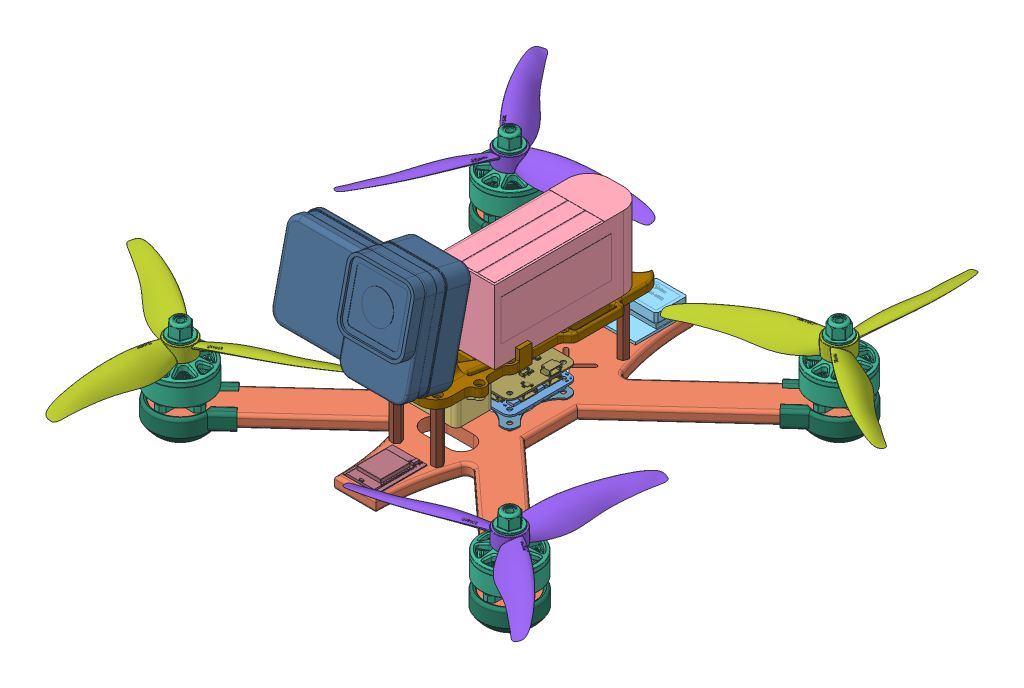
SolidWorks assembly Quad_assem, configuration Default. Lengths in mm.
Overall size (299.08 101.42 318.47).
26 component instances, 15 part files, 57 mates.
Components (placement in the parent):
- 4in1_ESC-1: 4in1_ESC [Default] at (-19.4317 14.4597 116.374) x (-1 0 0) z (0 1 0) size (33 33 7.6)
- Quad-1: Quad [Default] at (-19.4317 0 116.374) x (-1 0 0) z (0 0 -1) size (185.81 6.16 185.81)
- ToF-1: ToF [Default] at (-19.4317 31 146.374) x (1 0 0) z (0 0 -1) size (34.5 13.5 18.5)
- Battery-1: Battery [Default] at (-6 52.75 100.8519) x (0 0 1) z (-1 0 0) size (72.6 35.7 27.2)
- GPS_sam-m8q-2: GPS_sam-m8q [Default] at (-27.0434 7.25 37.7378) size (16.15 7.55 26.25)
- DYS SF2207 Motor.step-1: DYS SF2207 Motor.step [Default] at (60.4714 6 196.277) x (-0.126886 0 -0.991917) z (0.991917 0 -0.126886) size (27.7 33.34 27.7)
- DYS SF2207 Motor.step-2: DYS SF2207 Motor.step [Default] at (60.4714 6 36.4709) x (0.985702 0 -0.1685) z (0.1685 0 0.985702) size (27.7 33.34 27.7)
- DYS SF2207 Motor.step-3: DYS SF2207 Motor.step [Default] at (-99.3348 6 36.4709) x (0.155615 0 0.987818) z (-0.987818 0 0.155615) size (27.7 33.34 27.7)
- DYS SF2207 Motor.step-4: DYS SF2207 Motor.step [Default] at (-99.3348 6 196.277) x (0.148303 0 0.988942) z (-0.988942 0 0.148303) size (27.7 33.34 27.7)
- 50 Prop CW-1: 50 Prop CW [Default] at (60.4714 25.2 36.4709) x (-0.893778 0 0.44851) z (-0.44851 0 -0.893778) size (98.6 8.5 111.89)
- 50 Prop CCW-1: 50 Prop CCW [Default] at (2.1837 28.725 127.366) x (0.945285 0 -0.326246) z (0.326246 0 0.945285) size (98.59 8.5 111.89)
- 50 Prop CCW-2: 50 Prop CCW [Default] at (-50.9884 28.725 -39.7446) x (0.593794 0 0.804617) z (-0.804617 0 0.593794) size (98.59 8.5 111.89)
- 50 Prop CW-2: 50 Prop CW [Default] at (-99.3348 25.2 196.277) x (-0.021995 0 0.999758) z (-0.999758 0 -0.021995) size (98.6 8.5 111.89)
- Quad Top-1: Quad Top [Default] at (-19.4317 31 116.374) x (-1 0 0) z (0 0 -1) size (36.7 13 110.63)
- GOPRO_10_BONES-1: GOPRO_10_BONES [Default] at (-70.9317 42.3222 182.949) x (1 0 0) z (0 0.975758 -0.218854) size (68 37 50)
- Spacer-1: Spacer [Default] at (-9.4317 6 71.374) x (0.702092 0 0.712086) z (-0.712086 0 0.702092) size (5 25 4.33)
- Spacer-2: Spacer [Default] at (-29.4317 6 71.374) x (0.624402 0 0.781104) z (-0.781104 0 0.624402) size (5 25 4.33)
- Spacer-3: Spacer [Default] at (-9.4317 6 161.374) x (0.997584 0 -0.069465) z (0.069465 0 0.997584) size (5 25 4.33)
- Spacer-4: Spacer [Default] at (-29.4317 6 161.374) x (0.991206 0 0.132327) z (-0.132327 0 0.991206) size (5 25 4.33)
- FlightController-1: FlightController [Default] at (-19.4317 21.1634 116.374) x (-1 0 0) z (0 1 0) size (33 33.5 8.12)
- XBee_breakout-1: XBee_breakout [Default] at (-19.5608 6.4115 179.1808) x (-1 0 0) z (0 1 0) size (16.8 24.05 2.88)
- OpticalSensor.step-1: OpticalSensor.step [Default] at (-19.4317 8.6237 116.374) x (0 0 -1) z (0 1 0) size (33 33 6.87)
- Feet-1: Feet [Default] at (60.4714 -1 196.277) x (-0.999023 0 0.044203) z (-0.044203 0 -0.999023) size (35.07 16.09 35.07)
- Feet-2: Feet [Default] at (-99.3348 -1 36.4709) x (0.998911 0 -0.046652) z (0.046652 0 0.998911) size (35.07 16.09 35.07)
- Feet-3: Feet [Default] at (60.4714 -1 36.4709) x (-0.052266 0 0.998633) z (-0.998633 0 -0.052266) size (35.07 16.09 35.07)
- Feet-4: Feet [Default] at (-99.3348 -1 196.277) x (0.04359 0 -0.999049) z (0.999049 0 0.04359) size (35.07 16.09 35.07)
Mates (geometry in assembly coordinates):
- Distance6: distance = 6 mm aligned: plane of Battery-1 through (-6 52.75 100.8519) normal (1 0 0)
- Concentric5: concentric aligned: circle of 4in1_ESC-1; circle of Quad-1
- Concentric6: concentric aligned: circle of 4in1_ESC-1; circle of Quad-1
- Coincident38: coincident anti-aligned: plane of Quad-1 through (-99.3348 6 36.4709) normal (0 1 0); plane of DYS SF2207 Motor.step-1 through (64.4945 6 192.5268) normal (0 -1 0)
- Coincident39: coincident anti-aligned: plane of Quad-1 through (-99.3348 6 36.4709) normal (0 1 0); plane of DYS SF2207 Motor.step-2 through (64.3876 6 40.3327) normal (0 -1 0)
- Coincident40: coincident anti-aligned: plane of Quad-1 through (-99.3348 6 36.4709) normal (0 1 0); plane of DYS SF2207 Motor.step-3 through (-103.2474 6 40.3363) normal (0 -1 0)
- Coincident41: coincident anti-aligned: plane of Quad-1 through (-99.3348 6 36.4709) normal (0 1 0); plane of DYS SF2207 Motor.step-4 through (-103.2759 6 200.1134) normal (0 -1 0)
- Coincident42: coincident anti-aligned: plane of DYS SF2207 Motor.step-1 through (56.3233 25.2 192.978) normal (0 1 0); plane of 50 Prop CCW-1 through (60.4714 25.2 196.277) normal (0 -1 0)
- Coincident43: coincident anti-aligned: plane of DYS SF2207 Motor.step-3 through (-95.0927 25.2 39.6482) normal (0 1 0); plane of 50 Prop CCW-2 through (-99.3348 25.2 36.4709) normal (0 -1 0)
- Coincident44: coincident anti-aligned: plane of DYS SF2207 Motor.step-4 through (-95.1163 25.2 199.4856) normal (0 1 0); plane of 50 Prop CW-2 through (-99.3348 25.2 196.277) normal (0 -1 0)
- Coincident45: coincident anti-aligned: plane of DYS SF2207 Motor.step-2 through (63.593 25.2 32.1877) normal (0 1 0); plane of 50 Prop CW-1 through (60.4714 25.2 36.4709) normal (0 -1 0)
- Concentric15: concentric aligned: cylinder of DYS SF2207 Motor.step-1 through (60.4714 25.2 196.277) axis (0 1 0) radius 2.5; cylinder of 50 Prop CCW-1 through (60.4714 28.7 196.277) axis (0 1 0) radius 2.5
- Concentric16: concentric anti-aligned: cylinder of DYS SF2207 Motor.step-2 through (60.4714 25.2 36.4709) axis (0 1 0) radius 2.5; cylinder of 50 Prop CW-1 through (60.4714 28.7 36.4709) axis (0 -1 0) radius 2.5
- Concentric17: concentric aligned: cylinder of DYS SF2207 Motor.step-3 through (-99.3348 25.2 36.4709) axis (0 1 0) radius 2.5; cylinder of 50 Prop CCW-2 through (-99.3348 28.7 36.4709) axis (0 1 0) radius 2.5
- Concentric18: concentric anti-aligned: cylinder of DYS SF2207 Motor.step-4 through (-99.3348 25.2 196.277) axis (0 1 0) radius 2.5; cylinder of 50 Prop CW-2 through (-99.3348 28.7 196.277) axis (0 -1 0) radius 2.5
- Concentric19: concentric aligned: cylinder of DYS SF2207 Motor.step-3 through (-99.3348 25.2 36.4709) axis (0 1 0) radius 2.5; cylinder of 50 Prop CCW-2 through (-99.3348 28.7 36.4709) axis (0 1 0) radius 2.5
- Coincident53: coincident anti-aligned: plane of ToF-1 through (-8.7317 31 139.624) normal (0 1 0); plane of Quad Top-1 through (-4.1817 31 146.374) normal (0 -1 0)
- Concentric25: concentric aligned: circle of Quad-1; circle of Quad Top-1
- Concentric26: concentric aligned: circle of Quad-1; circle of Quad Top-1
- Coincident57: coincident anti-aligned: plane of Quad-1 through (-99.3348 0 36.4709) normal (0 -1 0)
- Coincident58: coincident anti-aligned: plane of Quad-1 through (-99.3348 6 36.4709) normal (0 1 0); plane of GPS_sam-m8q-2 through (-27.0434 6 37.7378) normal (0 -1 0)
- Parallel1: parallel aligned: plane of Quad-1 through (-10.4317 63.0088 36.374) normal (1 0 0); plane of GPS_sam-m8q-2 through (-11.2684 6 63.5878) normal (1 0 0)
- Concentric27: concentric aligned: circle of Quad-1; circle of DYS SF2207 Motor.step-1
- Concentric28: concentric aligned: circle of Quad-1; circle of DYS SF2207 Motor.step-4
- Concentric29: concentric aligned: circle of Quad-1; circle of DYS SF2207 Motor.step-3
- Concentric30: concentric aligned: circle of Quad-1; circle of DYS SF2207 Motor.step-2
- Concentric31: concentric anti-aligned: circle of Quad Top-1; circle of GOPRO_10_BONES-1
- Distance10: distance = 3 mm aligned: plane of GOPRO_10_BONES-1 through (-22.1817 38.2643 160.2878) normal (-1 0 0); plane of Quad Top-1 through (-25.1817 44 158.374) normal (-1 0 0)
- Concentric32: concentric aligned: circle of Quad-1; circle of Spacer-3
- Concentric33: concentric aligned: circle of Quad-1; circle of Spacer-1
- Concentric34: concentric aligned: circle of Quad-1; circle of Spacer-2
- Concentric35: concentric aligned: circle of Quad-1; circle of Spacer-4
- Coincident60: coincident anti-aligned: plane of Quad-1 through (-99.3348 6 36.4709) normal (0 1 0); plane of Spacer-2 through (-29.4317 6 71.374) normal (0 -1 0)
- Coincident61: coincident anti-aligned: plane of Quad-1 through (-99.3348 6 36.4709) normal (0 1 0); plane of Spacer-4 through (-29.4317 6 161.374) normal (0 -1 0)
- Coincident62: coincident anti-aligned: plane of Quad-1 through (-99.3348 6 36.4709) normal (0 1 0); plane of Spacer-3 through (-9.4317 6 161.374) normal (0 -1 0)
- Coincident63: coincident anti-aligned: plane of Quad-1 through (-99.3348 6 36.4709) normal (0 1 0); plane of Spacer-1 through (-9.4317 6 71.374) normal (0 -1 0)
- Distance13: distance = 6.08 mm anti-aligned: plane of FlightController-1 through (-19.4317 20.5397 116.374) normal (0 -1 0); plane of 4in1_ESC-1 through (-2.9317 14.4597 103.374) normal (0 1 0)
- Concentric42: concentric aligned: circle of 4in1_ESC-1; circle of FlightController-1
- Concentric43: concentric aligned: circle of 4in1_ESC-1; circle of FlightController-1
- Concentric44: concentric anti-aligned: circle of ToF-1; circle of Quad Top-1
- Concentric45: concentric anti-aligned: circle of ToF-1; circle of Quad Top-1
- Coincident78: coincident anti-aligned: plane of Quad-1 through (-99.3348 6 36.4709) normal (0 1 0); plane of XBee_breakout-1 through (-19.5608 6 176.8033) normal (0 -1 0)
- Coincident80: coincident anti-aligned: plane of Quad Top-1 through (-4.1817 31 146.374) normal (0 -1 0); plane of Spacer-3 through (-9.4317 31 161.374) normal (0 1 0)
- Coincident81: coincident anti-aligned: plane of Battery-1 through (-33 35 64.5519) normal (0 -1 0); plane of Quad Top-1 through (-4.1817 35 146.374) normal (0 1 0)
- Parallel6: parallel aligned: plane of XBee_breakout-1 through (-27.9608 6 188.8258) normal (-1 0 0); plane of Quad-1 through (-39.4317 231.245 103.485) normal (-1 0 0)
- Distance14: distance = 2 mm anti-aligned: plane of Quad-1 through (-99.3348 6 36.4709) normal (0 1 0); plane of OpticalSensor.step-1 through (-19.4317 8 116.374) normal (0 -1 0)
- Concentric47: concentric aligned: circle of Quad-1; circle of OpticalSensor.step-1
- Concentric48: concentric aligned: circle of Quad-1; circle of OpticalSensor.step-1
- Distance15: distance = 5 mm anti-aligned: plane of 4in1_ESC-1 through (-2.9317 13.6237 103.374) normal (0 -1 0); plane of OpticalSensor.step-1 through (-19.4317 8.6237 116.374) normal (0 1 0)
- Coincident82: coincident anti-aligned: plane of Quad-1 through (-99.3348 0 36.4709) normal (0 -1 0); plane of Feet-1 through (60.4714 0 196.277) normal (0 1 0)
- Concentric49: concentric anti-aligned: circle of Quad-1; circle of Feet-1
- Coincident84: coincident: plane of Quad-1 through (-99.3348 0 36.4709) normal (0 -1 0); plane of Feet-2 through (-99.3348 0 36.4709) normal (0 1 0)
- Coincident85: coincident: plane of Quad-1 through (-99.3348 0 36.4709) normal (0 -1 0); plane of Feet-3 through (60.4714 0 36.4709) normal (0 1 0)
- Coincident86: coincident: plane of Quad-1 through (-99.3348 0 36.4709) normal (0 -1 0); plane of Feet-4 through (-99.3348 0 196.277) normal (0 1 0)
- Concentric50: concentric anti-aligned: circle of Quad-1; circle of Feet-3
- Concentric51: concentric anti-aligned: circle of Quad-1; circle of Feet-4
- Concentric52: concentric anti-aligned: circle of Quad-1; circle of Feet-2
